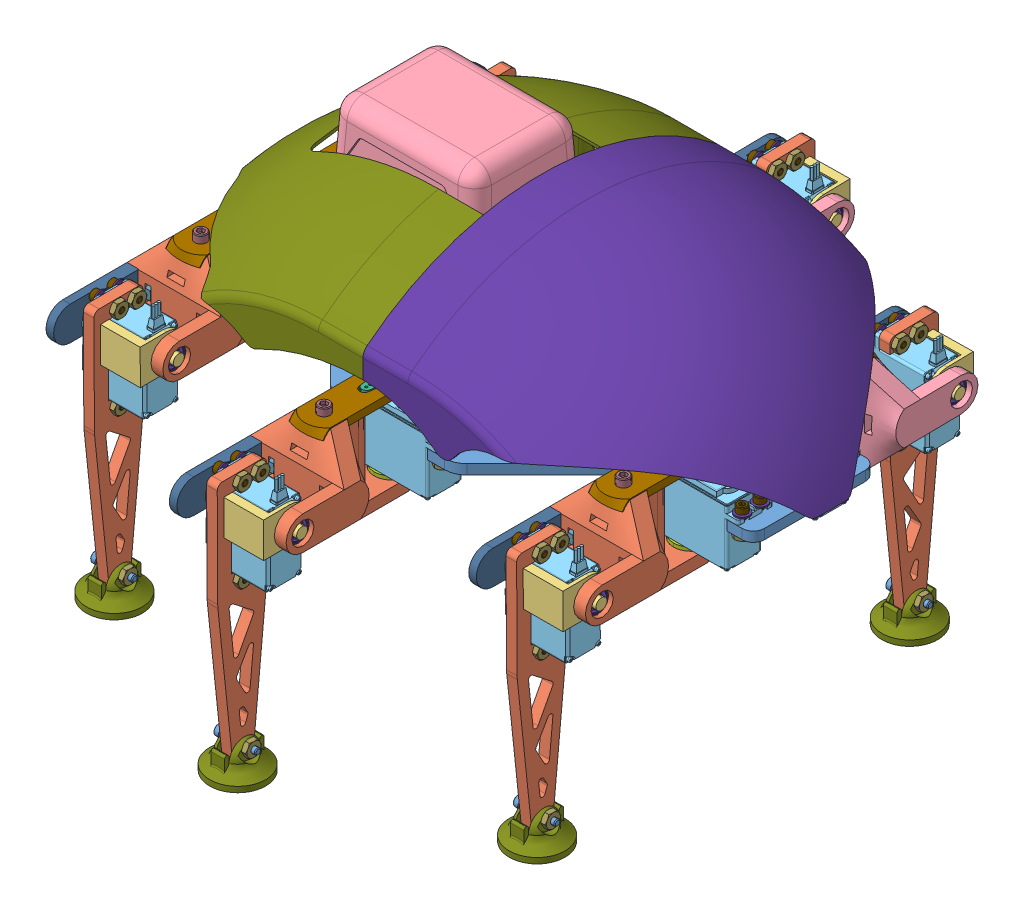
SolidWorks assembly Hexapod, configuration Défaut. Lengths in mm. (continued)
Mates (geometry in assembly coordinates): (continued)
- Concentric8: concentric aligned: cylinder of Body_V2-5 through (-298.75 -5.601 45.08) axis (0 1 0) radius 1.45; cylinder of Leg_(Straight_Foot)_(Mirror)-4/hs-422-3 through (-298.75 -26.67 45.08) axis (0 1 0) radius 2.1844
- Parallel7: parallel anti-aligned: plane of Body_V2-5 through (-295 -5.601 30) normal (0 0 1); plane of Leg_(Straight_Foot)_(Mirror)-4/hs-422-3 through (-275.001 -5.969 30.094) normal (0 0 -1)
- Coincident13: coincident anti-aligned: plane of Body_V2-5 through (-310 0 15) normal (0 1 0); plane of Leg_(Straight_Foot)_(Mirror)-5/hs-422-3 through (-35.001 0 49.906) normal (0 -1 0)
- Concentric9: concentric anti-aligned: cylinder of Body_V2-5 through (-58.75 0 45.08) axis (0 -1 0) radius 1.45; cylinder of Leg_(Straight_Foot)_(Mirror)-5/hs-422-3 through (-58.75 -26.67 45.08) axis (0 1 0) radius 2.1844
- Parallel8: parallel anti-aligned: plane of Body_V2-5 through (-55 -5.6 30) normal (0 0 1); plane of Leg_(Straight_Foot)_(Mirror)-5/hs-422-3 through (-35.001 -5.969 30.094) normal (0 0 -1)
- Coincident15: coincident anti-aligned: plane of Body_V2-5 through (-310 0 15) normal (0 1 0); plane of Leg_(Straight_Foot)_(Mirror)-6/hs-422-3 through (-155.001 0 99.906) normal (0 -1 0)
- Concentric10: concentric anti-aligned: cylinder of Body_V2-5 through (-178.75 0 95.08) axis (0 -1 0) radius 1.45; cylinder of Leg_(Straight_Foot)_(Mirror)-6/hs-422-3 through (-178.75 -26.67 95.08) axis (0 1 0) radius 2.1844
- Parallel9: parallel anti-aligned: plane of Body_V2-5 through (-175 -5.6 80) normal (0 0 1); plane of Leg_(Straight_Foot)_(Mirror)-6/hs-422-3 through (-155.001 -5.969 80.094) normal (0 0 -1)
- Coïncidente2: coincident anti-aligned: plane of arduinoMega-1 through (-199.11 -5.6 14.62) normal (0 1 0); plane of Body_V2-5 through (-310 -5.6 15) normal (0 -1 0)
- Coïncidente4: coincident anti-aligned: plane of Body_V2-5 through (-310 -5.6 15) normal (0 -1 0); plane of 12Channel PWM-1 through (-155 -5.6 -12.95) normal (0 1 0)
- Coïncidente5: coincident anti-aligned: plane of Body_V2-5 through (-310 -5.6 15) normal (0 -1 0); plane of DROK_090483.stp-1 through (-99 -5.6 15) normal (0 1 0)
- Parallèle4: parallel aligned: plane of Body_V2-5 through (0 0 50) normal (1 0 0); plane of 12Channel PWM-1 through (-132.9 -7.1 -12.95) normal (1 0 0)
- Concentric13: concentric aligned: cylinder of Body_V2-5 through (-155 0 42.95) axis (0 -1 0) radius 1.25; cylinder of 12Channel PWM-1 through (-155 -2.0645 42.95) axis (0 -1 0) radius 1.25
- Concentric17: concentric anti-aligned: circle of Body-1; circle of DROK_090483.stp-1
- Concentric18: concentric aligned: cylinder of Body_V2-5 through (-80.685 0 41.415) axis (0 -1 0) radius 1.45; cylinder of DROK_090483.stp-1 through (-80.685 -5.6 41.415) axis (0 -1 0) radius 1.585
- Concentric19: concentric aligned: cylinder of Body_V2-5 through (-175 0 -26) axis (0 -1 0) radius 1.6; circle of arduinoMega-1
- Concentric22: concentric aligned: cylinder of Body_V2-5 through (-223.22 0 50.11) axis (0 -1 0) radius 1.6; cylinder of arduinoMega-1 through (-223.22 -7.6 50.11) axis (0 -1 0) radius 1.6
- Concentric23: concentric anti-aligned: cylinder of Body_V2-5 through (-40.288 0 19.09) axis (0 -1 0) radius 1.45; cylinder of HX-SHCS 0.138-32x0.625x0.625-N-2 through (-40.288 35.2552 19.09) axis (0 1 0) radius 1.7526
- Concentric24: concentric anti-aligned: cylinder of Body_V2-5 through (-50.288 0 19.09) axis (0 -1 0) radius 1.45; cylinder of HX-SHCS 0.138-32x0.625x0.625-N-3 through (-50.288 35.2552 19.09) axis (0 1 0) radius 1.7526
- Coincident19: coincident anti-aligned: plane of Body_V2-5 through (-310 0 15) normal (0 1 0); plane of HX-SHCS 0.138-32x0.625x0.625-N-2 through (-40.288 0 16.2198) normal (0 -1 0)
- Coincident20: coincident anti-aligned: plane of Body_V2-5 through (-310 0 15) normal (0 1 0); plane of HX-SHCS 0.138-32x0.625x0.625-N-3 through (-47.8023 0 17.6549) normal (0 -1 0)
- Parallel10: parallel aligned: plane of Body_V2-5 through (0 0 50) normal (1 0 0); plane of HX-SHCS 0.138-32x0.625x0.625-N-3 through (-51.6723 1.8796 19.8892) normal (1 0 0)
- Parallel11: parallel aligned: plane of Body_V2-5 through (0 0 50) normal (1 0 0); plane of HX-SHCS 0.138-32x0.625x0.625-N-2 through (-41.6723 1.8796 18.2908) normal (1 0 0)
- Concentric25: concentric anti-aligned: cylinder of Body_V2-5 through (-50.288 0 10.91) axis (0 -1 0) radius 1.45; cylinder of HX-SHCS 0.138-32x0.625x0.625-N-4 through (-50.288 35.2552 10.91) axis (0 1 0) radius 1.7526
- Concentric26: concentric anti-aligned: cylinder of Body_V2-5 through (-40.288 0 10.91) axis (0 -1 0) radius 1.45; cylinder of HX-SHCS 0.138-32x0.625x0.625-N-5 through (-40.288 35.2552 10.91) axis (0 1 0) radius 1.7526
- Coincident23: coincident anti-aligned: plane of Body_V2-5 through (-310 0 15) normal (0 1 0); plane of HX-SHCS 0.138-32x0.625x0.625-N-5 through (-40.288 0 8.0398) normal (0 -1 0)
- Coincident24: coincident anti-aligned: plane of Body_V2-5 through (-310 0 15) normal (0 1 0); plane of HX-SHCS 0.138-32x0.625x0.625-N-4 through (-50.288 0 8.0398) normal (0 -1 0)
- Parallel12: parallel aligned: plane of Body_V2-5 through (0 0 50) normal (1 0 0); plane of HX-SHCS 0.138-32x0.625x0.625-N-5 through (-41.6723 1.8796 10.1108) normal (1 0 0)
- Parallel13: parallel aligned: plane of Body_V2-5 through (0 0 50) normal (1 0 0); plane of HX-SHCS 0.138-32x0.625x0.625-N-4 through (-51.6723 1.8796 10.1108) normal (1 0 0)
- Concentric27: concentric anti-aligned: cylinder of Body_(Small)-5 through (-170.288 0 -39.09) axis (0 -1 0) radius 1.45; cylinder of HX-SHCS 0.138-32x0.625x0.625-N-13 through (-214.94 40.2807 -39.09) axis (0 1 0) radius 1.7526
- Concentric29: concentric anti-aligned: cylinder of Body_V2-5 through (-160.288 0 69.09) axis (0 -1 0) radius 1.45; cylinder of HX-SHCS 0.138-32x0.625x0.625-N-7 through (-160.288 35.2552 69.09) axis (0 1 0) radius 1.7526
- Concentric30: concentric anti-aligned: cylinder of Body_V2-5 through (-170.288 0 69.09) axis (0 -1 0) radius 1.45; cylinder of HX-SHCS 0.138-32x0.625x0.625-N-6 through (-170.288 35.2552 69.09) axis (0 1 0) radius 1.7526
- Coincident27: coincident anti-aligned: plane of Body_V2-5 through (-310 0 15) normal (0 1 0); plane of HX-SHCS 0.138-32x0.625x0.625-N-7 through (-160.288 0 66.2198) normal (0 -1 0)
- Coincident28: coincident anti-aligned: plane of Body_V2-5 through (-310 0 15) normal (0 1 0); plane of HX-SHCS 0.138-32x0.625x0.625-N-6 through (-170.288 0 66.2198) normal (0 -1 0)
- Parallel14: parallel aligned: plane of Body_V2-5 through (0 0 50) normal (1 0 0); plane of HX-SHCS 0.138-32x0.625x0.625-N-6 through (-171.6723 1.8796 68.2908) normal (1 0 0)
- Parallel15: parallel aligned: plane of Body_V2-5 through (0 0 50) normal (1 0 0); plane of HX-SHCS 0.138-32x0.625x0.625-N-7 through (-161.6723 1.8796 68.2908) normal (1 0 0)
- Concentric31: concentric anti-aligned: cylinder of Body_V2-5 through (-170.288 0 -39.09) axis (0 -1 0) radius 1.45; cylinder of HX-SHCS 0.138-32x0.625x0.625-N-15 through (-170.288 35.2552 -39.09) axis (0 1 0) radius 1.7526
- Concentric32: concentric anti-aligned: cylinder of Body_V2-5 through (-160.288 0 -39.09) axis (0 -1 0) radius 1.45; cylinder of HX-SHCS 0.138-32x0.625x0.625-N-14 through (-160.288 35.2552 -39.09) axis (0 1 0) radius 1.7526
- Coincident31: coincident anti-aligned: plane of Body_V2-5 through (-310 0 15) normal (0 1 0); plane of HX-SHCS 0.138-32x0.625x0.625-N-15 through (-170.288 0 -41.9602) normal (0 -1 0)
- Coincident32: coincident anti-aligned: plane of Body_V2-5 through (-310 0 15) normal (0 1 0); plane of HX-SHCS 0.138-32x0.625x0.625-N-14 through (-160.288 0 -41.9602) normal (0 -1 0)
- Parallel16: parallel anti-aligned: plane of Body_V2-5 through (0 0 50) normal (1 0 0); plane of HX-SHCS 0.138-32x0.625x0.625-N-15 through (-168.9037 1.8796 -38.2908) normal (-1 0 0)
- Parallel17: parallel anti-aligned: plane of Body_V2-5 through (0 0 50) normal (1 0 0); plane of HX-SHCS 0.138-32x0.625x0.625-N-14 through (-158.9037 1.8796 -38.2908) normal (-1 0 0)
- Concentric33: concentric aligned: cylinder of Body_V2-5 through (-290.288 -5.601 19.09) axis (0 1 0) radius 1.45; cylinder of HX-SHCS 0.138-32x0.625x0.625-N-17 through (-290.288 35.2552 19.09) axis (0 1 0) radius 1.7526
- Concentric34: concentric aligned: circle of Body-1; cylinder of HX-SHCS 0.138-32x0.625x0.625-N-16 through (-280.288 35.2552 19.09) axis (0 1 0) radius 1.7526
- Concentric35: concentric aligned: cylinder of Body_V2-5 through (-290.288 -5.601 10.91) axis (0 1 0) radius 1.45; cylinder of HX-SHCS 0.138-32x0.625x0.625-N-18 through (-290.288 35.2552 10.91) axis (0 1 0) radius 1.7526
- Concentric36: concentric aligned: cylinder of Body_V2-5 through (-280.288 -5.601 10.91) axis (0 1 0) radius 1.45; cylinder of HX-SHCS 0.138-32x0.625x0.625-N-19 through (-280.288 35.2552 10.91) axis (0 1 0) radius 1.7526
- Coincident35: coincident anti-aligned: plane of Body_V2-5 through (-310 0 15) normal (0 1 0); plane of HX-SHCS 0.138-32x0.625x0.625-N-18 through (-290.288 0 8.0398) normal (0 -1 0)
- Coincident36: coincident anti-aligned: plane of Body_V2-5 through (-310 0 15) normal (0 1 0); plane of HX-SHCS 0.138-32x0.625x0.625-N-19 through (-280.288 0 8.0398) normal (0 -1 0)
- Coincident37: coincident anti-aligned: plane of Body_V2-5 through (-310 0 15) normal (0 1 0); plane of HX-SHCS 0.138-32x0.625x0.625-N-17 through (-287.8023 0 17.6549) normal (0 -1 0)
- Coincident38: coincident anti-aligned: plane of Body_V2-5 through (-310 0 15) normal (0 1 0); plane of HX-SHCS 0.138-32x0.625x0.625-N-16 through (-280.288 0 16.2198) normal (0 -1 0)
- Parallel18: parallel anti-aligned: plane of Body_V2-5 through (0 0 50) normal (1 0 0); plane of HX-SHCS 0.138-32x0.625x0.625-N-19 through (-278.9037 1.8796 11.7092) normal (-1 0 0)
- Parallel19: parallel anti-aligned: plane of Body_V2-5 through (0 0 50) normal (1 0 0); plane of HX-SHCS 0.138-32x0.625x0.625-N-18 through (-288.9037 1.8796 11.7092) normal (-1 0 0)
- Parallel20: parallel anti-aligned: plane of Body_V2-5 through (0 0 50) normal (1 0 0); plane of HX-SHCS 0.138-32x0.625x0.625-N-16 through (-278.9037 1.8796 19.8892) normal (-1 0 0)
- Parallel21: parallel anti-aligned: plane of Body_V2-5 through (0 0 50) normal (1 0 0); plane of HX-SHCS 0.138-32x0.625x0.625-N-17 through (-288.9037 1.8796 18.2908) normal (-1 0 0)
- Concentric37: concentric anti-aligned: cylinder of Leg_(Straight_Foot)-7/socket_1_2_6-32_with_washer-7/HX-SHCS 0.138-32x0.5x0.5-N-1 through (-298.75 38.5826 -15.08) axis (0 1 0) radius 1.7526; circle of MSHXNUT 0.138-32-D-N-1
- Coincident40: coincident anti-aligned: plane of Body_V2-5 through (-310 -5.6 15) normal (0 -1 0); plane of MSHXNUT 0.138-32-D-N-60 through (-306.6748 -5.6 -15.08) normal (0 1 0)
- Parallel22: parallel aligned: plane of Leg-7/hs-422-3 through (-294.94 -5.969 -0.094) normal (-1 0 0); plane of MSHXNUT 0.138-32-D-N-60 through (-302.7124 -5.6 -12.7923) normal (-1 0 0)
- Concentric38: concentric anti-aligned: cylinder of Leg_(Straight_Foot)-7/socket_1_2_6-32_with_washer-5/HX-SHCS 0.138-32x0.5x0.5-N-1 through (-298.75 38.5826 -4.92) axis (0 1 0) radius 1.7526; circle of MSHXNUT 0.138-32-D-N-2
- Parallel23: parallel aligned: plane of Leg-7/hs-422-3 through (-294.94 -5.969 -0.094) normal (-1 0 0); plane of MSHXNUT 0.138-32-D-N-65 through (-302.7124 -5.6 -2.6323) normal (-1 0 0)
- Coincident44: coincident anti-aligned: plane of Body_V2-5 through (-310 -5.6 15) normal (0 -1 0); plane of MSHXNUT 0.138-32-D-N-65 through (-306.6748 -5.6 -4.92) normal (0 1 0)
- Coincident45: coincident anti-aligned: cylinder of Leg_(Straight_Foot)-7/socket_1_2_6-32_with_washer-8/HX-SHCS 0.138-32x0.5x0.5-N-1 through (-251.252 38.5826 -4.92) axis (0 1 0) radius 1.7526; circle of MSHXNUT 0.138-32-D-N-3
- Concentric40: concentric anti-aligned: cylinder of Leg_(Straight_Foot)-7/socket_1_2_6-32_with_washer-6/HX-SHCS 0.138-32x0.5x0.5-N-1 through (-251.252 38.5826 -15.08) axis (0 1 0) radius 1.7526; circle of MSHXNUT 0.138-32-D-N-4
- Coincident47: coincident anti-aligned: plane of Body_V2-5 through (-310 -5.6 15) normal (0 -1 0); plane of MSHXNUT 0.138-32-D-N-75 through (-255.2144 -5.6 -21.9431) normal (0 1 0)
- Coincident48: coincident anti-aligned: plane of Body_V2-5 through (-310 -5.6 15) normal (0 -1 0); plane of MSHXNUT 0.138-32-D-N-70 through (-255.2144 -5.6 -11.7831) normal (0 1 0)
- Parallel24: parallel aligned: plane of Leg-7/hs-422-3 through (-255.062 -5.969 -0.094) normal (1 0 0); plane of MSHXNUT 0.138-32-D-N-75 through (-247.2896 -5.6 -17.3677) normal (1 0 0)
- Parallel25: parallel aligned: plane of Leg-7/hs-422-3 through (-255.062 -5.969 -0.094) normal (1 0 0); plane of MSHXNUT 0.138-32-D-N-70 through (-247.2896 -5.6 -7.2077) normal (1 0 0)
- Concentric41: concentric anti-aligned: cylinder of HX-SHCS 0.138-32x0.625x0.625-N-19 through (-280.288 35.2552 10.91) axis (0 1 0) radius 1.7526; circle of MSHXNUT 0.138-32-D-N-5
- Concentric42: concentric anti-aligned: cylinder of HX-SHCS 0.138-32x0.625x0.625-N-18 through (-290.288 35.2552 10.91) axis (0 1 0) radius 1.7526; circle of MSHXNUT 0.138-32-D-N-6
- Coincident53: coincident anti-aligned: plane of Leg-7/Bearing_mount_leg-1 through (-295.288 -10.67 15) normal (0 -1 0); plane of MSHXNUT 0.138-32-D-N-85 through (-290.288 -10.67 2.9852) normal (0 1 0)
- Coincident54: coincident anti-aligned: plane of Leg-7/Bearing_mount_leg-1 through (-295.288 -10.67 15) normal (0 -1 0); plane of MSHXNUT 0.138-32-D-N-80 through (-280.288 -10.67 2.9852) normal (0 1 0)
- Parallel26: parallel aligned: plane of Leg-7/Bearing_mount_leg-1 through (-295.288 -26.67 5) normal (0 0 1); plane of MSHXNUT 0.138-32-D-N-80 through (-282.5757 -10.67 14.8724) normal (0 0 1)
- Parallel27: parallel aligned: plane of Leg-7/Bearing_mount_leg-1 through (-295.288 -26.67 5) normal (0 0 1); plane of MSHXNUT 0.138-32-D-N-85 through (-292.5757 -10.67 14.8724) normal (0 0 1)
- Concentric43: concentric aligned: cylinder of arduinoMega-1 through (-175 -7.6 48.88) axis (0 -1 0) radius 1.6; cylinder of HX-SHCS 0.138-32x0.5x0.5-N-20 through (-175 -44.3552 48.88) axis (0 -1 0) radius 1.7526
- Concentric44: concentric aligned: cylinder of arduinoMega-1 through (-223.22 -7.6 50.11) axis (0 -1 0) radius 1.6; cylinder of HX-SHCS 0.138-32x0.5x0.5-N-23 through (-223.22 -44.3552 50.11) axis (0 -1 0) radius 1.7526
- Concentric45: concentric aligned: cylinder of arduinoMega-1 through (-223.22 -7.6 -32.36) axis (0 -1 0) radius 1.6; cylinder of HX-SHCS 0.138-32x0.5x0.5-N-21 through (-223.22 -44.3552 -32.36) axis (0 -1 0) radius 1.7526
- Concentric46: concentric aligned: cylinder of arduinoMega-1 through (-175 -7.6 -26) axis (0 -1 0) radius 1.6; cylinder of HX-SHCS 0.138-32x0.5x0.5-N-22 through (-175 -44.3552 -26) axis (0 -1 0) radius 1.7526
- Coincident58: coincident anti-aligned: plane of arduinoMega-1 through (-199.11 -9.1 14.62) normal (0 -1 0); plane of HX-SHCS 0.138-32x0.5x0.5-N-20 through (-172.5143 -9.1 47.4449) normal (0 1 0)
- Coincident59: coincident anti-aligned: plane of arduinoMega-1 through (-199.11 -9.1 14.62) normal (0 -1 0); plane of HX-SHCS 0.138-32x0.5x0.5-N-22 through (-172.5143 -9.1 -27.4351) normal (0 1 0)
- Coincident60: coincident anti-aligned: plane of arduinoMega-1 through (-199.11 -9.1 14.62) normal (0 -1 0); plane of HX-SHCS 0.138-32x0.5x0.5-N-23 through (-223.22 -9.1 47.2398) normal (0 1 0)
- Coincident61: coincident anti-aligned: plane of arduinoMega-1 through (-199.11 -9.1 14.62) normal (0 -1 0); plane of HX-SHCS 0.138-32x0.5x0.5-N-21 through (-223.22 -9.1 -29.4898) normal (0 1 0)
- Concentric47: concentric anti-aligned: cylinder of HX-SHCS 0.138-32x0.5x0.5-N-21 through (-223.22 -44.3552 -32.36) axis (0 -1 0) radius 1.7526; circle of MSHXNUT 0.112-40-S-N-2
- Concentric48: concentric anti-aligned: cylinder of HX-SHCS 0.138-32x0.5x0.5-N-23 through (-223.22 -44.3552 50.11) axis (0 -1 0) radius 1.7526; circle of MSHXNUT 0.112-40-S-N-3
- Concentric49: concentric anti-aligned: cylinder of HX-SHCS 0.138-32x0.5x0.5-N-22 through (-175 -44.3552 -26) axis (0 -1 0) radius 1.7526; circle of MSHXNUT 0.112-40-S-N-4
- Concentric50: concentric anti-aligned: cylinder of HX-SHCS 0.138-32x0.5x0.5-N-20 through (-175 -44.3552 48.88) axis (0 -1 0) radius 1.7526; circle of MSHXNUT 0.112-40-S-N-5
- Coincident62: coincident anti-aligned: plane of Body_V2-5 through (-310 0 15) normal (0 1 0); plane of MSHXNUT 0.112-40-D-N-109 through (-181.35 0 48.88) normal (0 -1 0)
- Coincident63: coincident anti-aligned: plane of Body_V2-5 through (-310 0 15) normal (0 1 0); plane of MSHXNUT 0.112-40-D-N-108 through (-181.35 0 -26) normal (0 -1 0)
- Coincident64: coincident anti-aligned: plane of Body_V2-5 through (-310 0 15) normal (0 1 0); plane of MSHXNUT 0.112-40-D-N-107 through (-229.57 0 50.11) normal (0 -1 0)
- Coincident65: coincident anti-aligned: plane of Body_V2-5 through (-310 0 15) normal (0 1 0); plane of MSHXNUT 0.112-40-D-N-106 through (-229.57 0 -32.36) normal (0 -1 0)
- Parallel28: parallel anti-aligned: plane of Body_V2-5 through (-310 0 15) normal (-1 0 0); plane of MSHXNUT 0.112-40-D-N-107 through (-220.045 0 48.2769) normal (1 0 0)
- Parallel30: parallel aligned: plane of Body_V2-5 through (-310 0 15) normal (-1 0 0); plane of MSHXNUT 0.112-40-D-N-106 through (-226.395 0 -34.1931) normal (-1 0 0)
- Parallel31: parallel aligned: plane of Body_V2-5 through (-310 0 15) normal (-1 0 0); plane of MSHXNUT 0.112-40-D-N-108 through (-178.175 0 -27.8331) normal (-1 0 0)
- Parallel32: parallel aligned: plane of Body_V2-5 through (-310 0 15) normal (-1 0 0); plane of MSHXNUT 0.112-40-D-N-109 through (-178.175 0 47.0469) normal (-1 0 0)
- Parallel33: parallel aligned: plane of arduinoMega-1 through (-225.76 -9.1 64.11) normal (-1 0 0); plane of HX-SHCS 0.138-32x0.5x0.5-N-23 through (-221.8357 -10.9796 49.3108) normal (-1 0 0)
- Parallel34: parallel aligned: plane of arduinoMega-1 through (-225.76 -9.1 64.11) normal (-1 0 0); plane of HX-SHCS 0.138-32x0.5x0.5-N-20 through (-173.6157 -10.9796 48.0808) normal (-1 0 0)
- Parallel35: parallel aligned: plane of arduinoMega-1 through (-225.76 -9.1 64.11) normal (-1 0 0); plane of HX-SHCS 0.138-32x0.5x0.5-N-22 through (-173.6157 -10.9796 -26.7992) normal (-1 0 0)
- Parallel36: parallel aligned: plane of arduinoMega-1 through (-225.76 -9.1 64.11) normal (-1 0 0); plane of HX-SHCS 0.138-32x0.5x0.5-N-21 through (-221.8357 -10.9796 -33.1592) normal (-1 0 0)
- Concentric51: concentric aligned: cylinder of DROK_090483.stp-1 through (-117.315 -5.6 -11.415) axis (0 -1 0) radius 1.585; cylinder of HX-SHCS 0.138-32x0.5x0.5-N-24 through (-117.315 -42.0552 -11.415) axis (0 -1 0) radius 1.7526
- Coincident74: coincident anti-aligned: plane of DROK_090483.stp-1 through (-99 -6.8 15) normal (0 -1 0); plane of HX-SHCS 0.138-32x0.5x0.5-N-24 through (-114.8293 -6.8 -12.8501) normal (0 1 0)
- Parallel37: parallel aligned: plane of DROK_090483.stp-1 through (-120.5 -5.6 45) normal (-1 0 0); plane of HX-SHCS 0.138-32x0.5x0.5-N-24 through (-115.9307 -8.6796 -12.2142) normal (-1 0 0)
- Concentric52: concentric anti-aligned: cylinder of HX-SHCS 0.138-32x0.5x0.5-N-24 through (-117.315 -42.0552 -11.415) axis (0 -1 0) radius 1.7526; circle of MSHXNUT 0.112-40-S-N-6
- Coincident76: coincident anti-aligned: plane of Body_V2-5 through (-310 0 15) normal (0 1 0); plane of MSHXNUT 0.112-40-D-N-110 through (-123.665 0 -11.415) normal (0 -1 0)
- Parallel38: parallel anti-aligned: plane of Body_V2-5 through (0 0 50) normal (1 0 0); plane of MSHXNUT 0.112-40-D-N-110 through (-120.49 0 -13.2481) normal (-1 0 0)
- Concentric53: concentric anti-aligned: cylinder of Body_V2-5 through (-70 -5.6 -9.5) axis (0 1 0) radius 1.375; cylinder of 1_4_Round_Aluminum_Standoff.step-1 through (-70 6.35 -9.5) axis (0 -1 0) radius 3.1712
- Coincident78: coincident anti-aligned: plane of Body_V2-5 through (-310 0 15) normal (0 1 0); plane of 1_4_Round_Aluminum_Standoff.step-1 through (-70 0 -9.5) normal (0 -1 0)
- Coincident83: coincident anti-aligned: plane of Body_V2-5 through (-310 -5.6 15) normal (0 -1 0); plane of MSHXNUT 0.112-40-D-N-117 through (-76.35 -5.6 -9.5) normal (0 1 0)
- Parallel40: parallel aligned: plane of Body_V2-5 through (0 0 50) normal (1 0 0); plane of MSHXNUT 0.112-40-D-N-117 through (-66.825 -5.6 -7.6669) normal (1 0 0)
- Concentric56: concentric aligned: cylinder of 12Channel PWM-1 through (-155 -2.0645 -12.95) axis (0 -1 0) radius 1.25; cylinder of HX-SHCS 0.112-40x0.5x0.5-N-32 through (-155 -41.6948 -12.95) axis (0 -1 0) radius 1.4224
- Coincident85: coincident anti-aligned: plane of 12Channel PWM-1 through (-155 -7.1 -12.95) normal (0 -1 0); plane of HX-SHCS 0.112-40x0.5x0.5-N-32 through (-155 -7.1 -15.2741) normal (0 1 0)
- Parallel41: parallel aligned: plane of 12Channel PWM-1 through (-132.9 -7.1 -12.95) normal (1 0 0); plane of HX-SHCS 0.112-40x0.5x0.5-N-32 through (-156.1938 -8.6494 -12.2608) normal (1 0 0)
- Concentric57: concentric anti-aligned: cylinder of HX-SHCS 0.112-40x0.5x0.5-N-32 through (-155 -41.6948 -12.95) axis (0 -1 0) radius 1.4224; circle of MSHXNUT 0.112-40-D-N-68
- Coincident88: coincident anti-aligned: plane of Body_V2-5 through (-310 0 15) normal (0 1 0); plane of MSHXNUT 0.112-40-D-N-124 through (-161.35 0 -12.95) normal (0 -1 0)
- Parallel42: parallel aligned: plane of Body_V2-5 through (0 0 50) normal (1 0 0); plane of MSHXNUT 0.112-40-D-N-124 through (-151.825 0 -14.7831) normal (1 0 0)
- Parallel43: parallel aligned: plane of raspberryPi3B-1 through (-66.5 7.65 43) normal (1 0 0); plane of Body_V2-5 through (0 0 50) normal (1 0 0)
- Concentric64: concentric aligned: circle of raspberryPi3B-1; cylinder of socket head cap screw_ai-65 through (-70 42.2448 -9.5) axis (0 1 0) radius 1.4224
- Coincident92: coincident aligned: cylinder of socket head cap screw_ai-65 through (-70 42.2448 -9.5) axis (0 1 0) radius 1.4224; circle of machine screw nut hex_ai-114
- Concentric65: concentric anti-aligned: cylinder of 1_4_Round_Aluminum_Standoff.step-3 through (-70 6.35 39.5) axis (0 -1 0) radius 3.1712; cylinder of HX-SHCS 0.112-40x1x0.75-N-70 through (-70 42.2448 39.5) axis (0 1 0) radius 1.4224
- Coincident93: coincident anti-aligned: plane of raspberryPi3B-1 through (-109 6.35 15) normal (0 -1 0); plane of 1_4_Round_Aluminum_Standoff.step-1 through (-70 6.35 -9.5) normal (0 1 0)
- Coincident96: coincident anti-aligned: plane of raspberryPi3B-1 through (-109 7.65 15) normal (0 1 0); plane of socket head cap screw_ai-65 through (-68.2097 7.65 -10.9819) normal (0 -1 0)
- Coincident97: coincident anti-aligned: plane of Body_V2-5 through (-310 0 15) normal (0 1 0); plane of 1_4_Round_Aluminum_Standoff.step-5 through (-174 0 -7) normal (0 -1 0)
- Concentric66: concentric aligned: cylinder of Body_V2-5 through (-174 4.1012 -7) axis (0 -1 0) radius 1.45; cylinder of 1_4_Round_Aluminum_Standoff.step-5 through (-174 6.35 -7) axis (0 -1 0) radius 3.1712
- Concentric68: concentric aligned: cylinder of 1_4_Round_Aluminum_Standoff.step-5 through (-174 6.35 -7) axis (0 -1 0) radius 3.1712; cylinder of HX-SHCS 0.112-40x1x0.75-N-72 through (-174 -40.1948 -7) axis (0 -1 0) radius 1.4224
- Coincident99: coincident anti-aligned: plane of Body_V2-5 through (-310 -5.6 15) normal (0 -1 0); plane of HX-SHCS 0.112-40x1x0.75-N-72 through (-171.8858 -5.6 -7.9652) normal (0 1 0)
- Coincident100: coincident anti-aligned: plane of 1_4_Round_Aluminum_Standoff.step-5 through (-174 6.35 -7) normal (0 1 0); plane of Batterie_holder-1 through (-191 6.35 30) normal (0 -1 0)
- Concentric69: concentric anti-aligned: cylinder of HX-SHCS 0.112-40x1x0.75-N-77 through (-240 -40.1948 -7) axis (0 -1 0) radius 1.4224; circle of Batterie_holder-1
- Concentric70: concentric anti-aligned: cylinder of HX-SHCS 0.112-40x1x0.75-N-76 through (-174 -40.1948 37) axis (0 -1 0) radius 1.4224; circle of Batterie_holder-1
- Coincident101: coincident anti-aligned: plane of Batterie_holder-1 through (-191 12.7 26) normal (0 1 0); plane of MSHXNUT 0.112-40-D-N-131 through (-180.35 12.7 -7) normal (0 -1 0)
- Coincident102: coincident anti-aligned: cylinder of HX-SHCS 0.112-40x1x0.75-N-72 through (-174 -40.1948 -7) axis (0 -1 0) radius 1.4224; circle of machine screw nut hex_ai-122
- Coincident103: coincident anti-aligned: plane of Battery-1/MAKITA 4.0AH MOBILE-1 through (-236.7799 25.95 32.4375) normal (0 -1 0); plane of Batterie_holder-1 through (-191 25.95 30) normal (0 1 0)
- Parallel45: parallel anti-aligned: plane of Battery-1/MAKITA 4.0AH MOBILE-1 through (-209.9758 102.15 37.2) normal (0 0 1); plane of Batterie_holder-1 through (-191 6.35 0) normal (0 0 -1)
- Distance2: distance = 1.5 mm anti-aligned: plane of Batterie_holder-1 through (-191 12.7 26) normal (0 0 -1); plane of Battery-1/MAKITA 4.0AH MOBILE-1 through (-223.3759 24.3052 24.5) normal (0 0 1)
- Distance3: distance = 6.1569 mm: line of Battery-1/MAKITA 4.0AH MOBILE-1 through (-226.6169 25.95 23.7062) axis (0 0 -1); line of Batterie_holder-1 through (-220.46 25.95 2.54) axis (0 0 1)
- Coincident109: coincident anti-aligned: plane of Body_V2-5 through (-310 0 15) normal (0 1 0); plane of Shell_front-3 through (-339.15 0 173.75) normal (0 -1 0)
- Concentric71: concentric aligned: circle of Body_V2-5; circle of Shell_front-2
- Concentric72: concentric anti-aligned: circle of Body_V2-5; circle of Shell_front-2
- Coincident112: coincident anti-aligned: plane of Body_V2-5 through (-310 0 15) normal (0 1 0); plane of Shell_back-3 through (29.15 0 -143.75) normal (0 -1 0)
- Concentric73: concentric aligned: circle of Body_V2-5; circle of Shell_back-3
- Concentric74: concentric anti-aligned: circle of Body_V2-5; circle of Shell_back-3
- Concentric75: concentric aligned: cylinder of Shell_(Back)-3 through (-114.1421 0 80) axis (0 1 0) radius 1.45; cylinder of HX-SHCS 0.138-32x0.625x0.625-N-20 through (-114.1421 41.6052 80) axis (0 1 0) radius 1.7526
- Coincident113: coincident anti-aligned: plane of Shell_(Back)-3 through (-155 6.35 15) normal (0 1 0); plane of HX-SHCS 0.138-32x0.625x0.625-N-20 through (-111.7393 6.35 81.5698) normal (0 -1 0)
- Concentric76: concentric anti-aligned: cylinder of HX-SHCS 0.138-32x0.625x0.625-N-20 through (-114.1421 41.6052 80) axis (0 1 0) radius 1.7526; cylinder of MSHXNUT 0.138-32-D-N-118 through (-114.1421 -5.6 80) axis (0 -1 0) radius 1.3526
- Coincident114: coincident anti-aligned: plane of Body_(Small)-5 through (-310 -5.6 15) normal (0 -1 0); plane of MSHXNUT 0.138-32-D-N-118 through (-118.1045 -5.6 73.1369) normal (0 1 0)
- Parallel46: parallel anti-aligned: plane of Leg_(Straight_Foot)_(Mirror)-6/hs-422-3 through (-135.062 -5.969 99.906) normal (1 0 0); plane of MSHXNUT 0.138-32-D-N-118 through (-118.1045 -5.6 82.2877) normal (-1 0 0)
